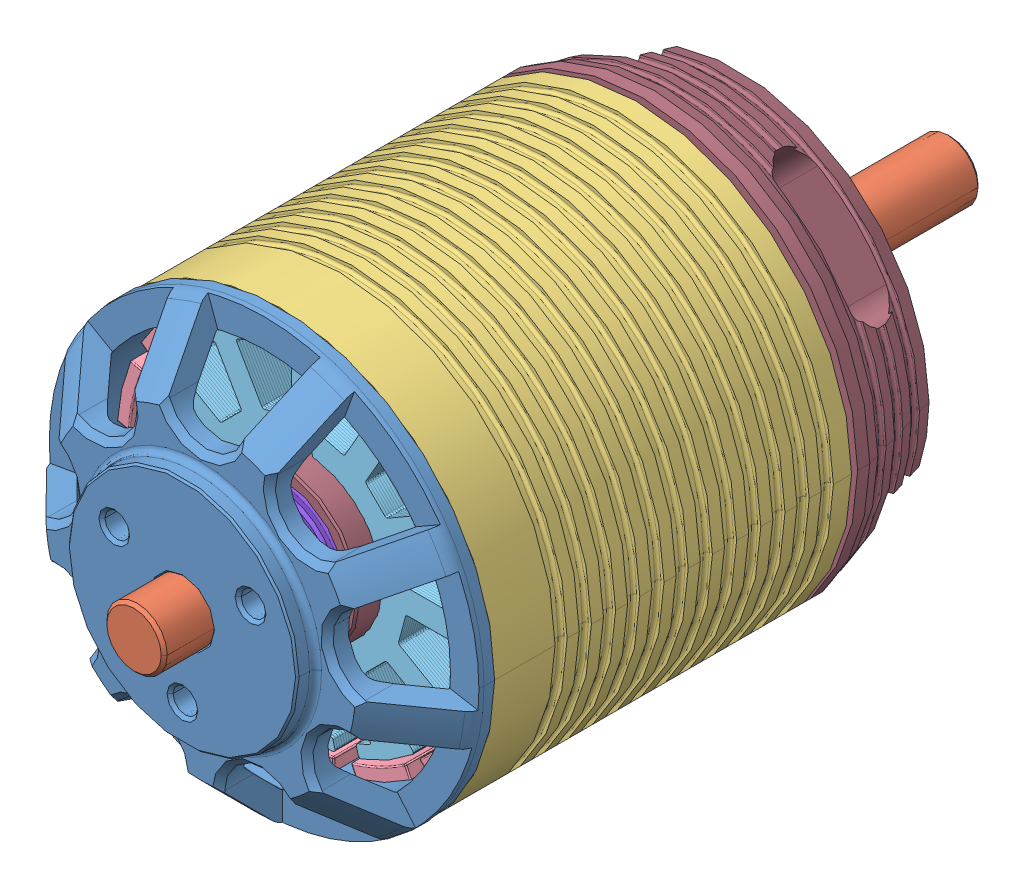
SolidWorks assembly BA-2826-Motor, configuration Default. Lengths in mm.
Overall size (35.6 35.6 67.5).
198 component instances, 15 part files, 0 mates.
Components (placement in the parent):
- BA-2826-Motor(2)^BA-2826-Motor-1: BA-2826-Motor(2)^BA-2826-Motor [Default] at origin size (35.6 35.6 67.5) (virtual)
  - 2826-Rotor-Assem^BA-2826-Motor(2)_BA-2826-Motor-1: 2826-Rotor-Assem^BA-2826-Motor(2)_BA-2826-Motor [Default] at (-10.2441 1.2166 27.3291) size (35.6 35.6 67.5) (virtual)
    - 28mm-Endbell-9^2826-Rotor-Assem_BA-2826-Motor(2)_BA-2826-Motor-1: 28mm-Endbell-9^2826-Rotor-Assem_BA-2826-Motor(2)_BA-2826-Motor [Default] at (-25.4444 8.584 0.3449) size (35.6 35.6 14.5) (virtual)
    - 2826-Shaft^2826-Rotor-Assem_BA-2826-Motor(2)_BA-2826-Motor-1: 2826-Shaft^2826-Rotor-Assem_BA-2826-Motor(2)_BA-2826-Motor [Default] at (-25.4444 8.584 -48.6551) size (5 5 67.5) (virtual)
    - 2826-Fluxring^2826-Rotor-Assem_BA-2826-Motor(2)_BA-2826-Motor-1: 2826-Fluxring^2826-Rotor-Assem_BA-2826-Motor(2)_BA-2826-Motor [Default] at (-25.4444 8.584 -22.6551) size (35.6 35.6 29.5) (virtual)
    - 2826-Magnet^2826-Rotor-Assem_BA-2826-Motor(2)_BA-2826-Motor-1: 2826-Magnet^2826-Rotor-Assem_BA-2826-Motor(2)_BA-2826-Motor [Default] at (-25.4444 8.584 -21.1551) size (5 2.2 26) (virtual)
    - 2826-Magnet^2826-Rotor-Assem_BA-2826-Motor(2)_BA-2826-Motor-2: 2826-Magnet^2826-Rotor-Assem_BA-2826-Motor(2)_BA-2826-Motor [Default] at (-25.4444 8.584 -21.1551) x (0.900969 0.433884 0) z (0 0 1) size (5 2.2 26) (virtual)
    - 2826-Magnet^2826-Rotor-Assem_BA-2826-Motor(2)_BA-2826-Motor-3: 2826-Magnet^2826-Rotor-Assem_BA-2826-Motor(2)_BA-2826-Motor [Default] at (-25.4444 8.584 -21.1551) x (0.62349 0.781831 0) z (0 0 1) size (5 2.2 26) (virtual)
    - 2826-Magnet^2826-Rotor-Assem_BA-2826-Motor(2)_BA-2826-Motor-4: 2826-Magnet^2826-Rotor-Assem_BA-2826-Motor(2)_BA-2826-Motor [Default] at (-25.4444 8.584 -21.1551) x (0.222521 0.974928 0) z (0 0 1) size (5 2.2 26) (virtual)
    - 2826-Magnet^2826-Rotor-Assem_BA-2826-Motor(2)_BA-2826-Motor-5: 2826-Magnet^2826-Rotor-Assem_BA-2826-Motor(2)_BA-2826-Motor [Default] at (-25.4444 8.584 -21.1551) x (-0.222521 0.974928 0) z (0 0 1) size (5 2.2 26) (virtual)
    - 2826-Magnet^2826-Rotor-Assem_BA-2826-Motor(2)_BA-2826-Motor-6: 2826-Magnet^2826-Rotor-Assem_BA-2826-Motor(2)_BA-2826-Motor [Default] at (-25.4444 8.584 -21.1551) x (-0.62349 0.781831 0) z (0 0 1) size (5 2.2 26) (virtual)
    - 2826-Magnet^2826-Rotor-Assem_BA-2826-Motor(2)_BA-2826-Motor-7: 2826-Magnet^2826-Rotor-Assem_BA-2826-Motor(2)_BA-2826-Motor [Default] at (-25.4444 8.584 -21.1551) x (-0.900969 0.433884 0) z (0 0 1) size (5 2.2 26) (virtual)
    - 2826-Magnet^2826-Rotor-Assem_BA-2826-Motor(2)_BA-2826-Motor-8: 2826-Magnet^2826-Rotor-Assem_BA-2826-Motor(2)_BA-2826-Motor [Default] at (-25.4444 8.584 -21.1551) x (-1 0 0) z (0 0 1) size (5 2.2 26) (virtual)
    - 2826-Magnet^2826-Rotor-Assem_BA-2826-Motor(2)_BA-2826-Motor-9: 2826-Magnet^2826-Rotor-Assem_BA-2826-Motor(2)_BA-2826-Motor [Default] at (-25.4444 8.584 -21.1551) x (-0.900969 -0.433884 0) z (0 0 1) size (5 2.2 26) (virtual)
    - 2826-Magnet^2826-Rotor-Assem_BA-2826-Motor(2)_BA-2826-Motor-10: 2826-Magnet^2826-Rotor-Assem_BA-2826-Motor(2)_BA-2826-Motor [Default] at (-25.4444 8.584 -21.1551) x (-0.62349 -0.781831 0) z (0 0 1) size (5 2.2 26) (virtual)
    - 2826-Magnet^2826-Rotor-Assem_BA-2826-Motor(2)_BA-2826-Motor-11: 2826-Magnet^2826-Rotor-Assem_BA-2826-Motor(2)_BA-2826-Motor [Default] at (-25.4444 8.584 -21.1551) x (-0.222521 -0.974928 0) z (0 0 1) size (5 2.2 26) (virtual)
    - 2826-Magnet^2826-Rotor-Assem_BA-2826-Motor(2)_BA-2826-Motor-12: 2826-Magnet^2826-Rotor-Assem_BA-2826-Motor(2)_BA-2826-Motor [Default] at (-25.4444 8.584 -21.1551) x (0.222521 -0.974928 0) z (0 0 1) size (5 2.2 26) (virtual)
    - 2826-Magnet^2826-Rotor-Assem_BA-2826-Motor(2)_BA-2826-Motor-13: 2826-Magnet^2826-Rotor-Assem_BA-2826-Motor(2)_BA-2826-Motor [Default] at (-25.4444 8.584 -21.1551) x (0.62349 -0.781831 0) z (0 0 1) size (5 2.2 26) (virtual)
    - 2826-Magnet^2826-Rotor-Assem_BA-2826-Motor(2)_BA-2826-Motor-14: 2826-Magnet^2826-Rotor-Assem_BA-2826-Motor(2)_BA-2826-Motor [Default] at (-25.4444 8.584 -21.1551) x (0.900969 -0.433884 0) z (0 0 1) size (5 2.2 26) (virtual)
  - 2826-Stator-Mount^BA-2826-Motor(2)_BA-2826-Motor-1: 2826-Stator-Mount^BA-2826-Motor(2)_BA-2826-Motor [Default] at (-12.4646 -13.2477 18.5701) size (35.6 35.6 38.01) (virtual)
    - 28x13x26mm-Stator^2826-Stator-Mount_BA-2826-Motor(2)_BA-2826-Motor-1: 28x13x26mm-Stator^2826-Stator-Mount_BA-2826-Motor(2)_BA-2826-Motor [Default] at (-35.5349 -3.2376 -36.4185) size (28 28 26) (virtual)
      - 28x13x5mm-Stator^28x13x26mm-Stator_2826-Stator-Mount_BA-2826-Motor(2)_BA-2826-Motor-1: 28x13x5mm-Stator^28x13x26mm-Stator_2826-Stator-Mount_BA-2826-Motor(2)_BA-2826-Motor [Default] at (6.5198 12.3714 25.0893) size (28 28 5) (virtual)
        - 28x13x1mm-Stator^28x13x5mm-Stator_28x13x26mm-Stator_2826-Stator-Mount_BA-2826-Motor(2)_BA-2826-Motor-1: 28x13x1mm-Stator^28x13x5mm-Stator_28x13x26mm-Stator_2826-Stator-Mount_BA-2826-Motor(2)_BA-2826-Motor [Default] at (34.0086 1.4103 18.4307) size (28 28 1) (virtual)
          - 28x13-Stator Plate^28x13x1mm-Stator_28x13x5mm-Stator_28x13x26mm-Stator_2826-Stator-Mount_BA-2826-Motor(2)_BA-2826-Motor-1: 28x13-Stator Plate^28x13x1mm-Stator_28x13x5mm-Stator_28x13x26mm-Stator_2826-Stator-Mount_BA-2826-Motor(2)_BA-2826-Motor [Default] at (-28.2175 12.5042 6.2948) size (28 28 0.2) (virtual)
          - 28x13-Stator Plate^28x13x1mm-Stator_28x13x5mm-Stator_28x13x26mm-Stator_2826-Stator-Mount_BA-2826-Motor(2)_BA-2826-Motor-2: 28x13-Stator Plate^28x13x1mm-Stator_28x13x5mm-Stator_28x13x26mm-Stator_2826-Stator-Mount_BA-2826-Motor(2)_BA-2826-Motor [Default] at (-28.2175 12.5042 6.0948) size (28 28 0.2) (virtual)
          - 28x13-Stator Plate^28x13x1mm-Stator_28x13x5mm-Stator_28x13x26mm-Stator_2826-Stator-Mount_BA-2826-Motor(2)_BA-2826-Motor-3: 28x13-Stator Plate^28x13x1mm-Stator_28x13x5mm-Stator_28x13x26mm-Stator_2826-Stator-Mount_BA-2826-Motor(2)_BA-2826-Motor [Default] at (-28.2175 12.5042 5.8948) size (28 28 0.2) (virtual)
          - 28x13-Stator Plate^28x13x1mm-Stator_28x13x5mm-Stator_28x13x26mm-Stator_2826-Stator-Mount_BA-2826-Motor(2)_BA-2826-Motor-4: 28x13-Stator Plate^28x13x1mm-Stator_28x13x5mm-Stator_28x13x26mm-Stator_2826-Stator-Mount_BA-2826-Motor(2)_BA-2826-Motor [Default] at (-28.2175 12.5042 5.6948) size (28 28 0.2) (virtual)
          - 28x13-Stator Plate^28x13x1mm-Stator_28x13x5mm-Stator_28x13x26mm-Stator_2826-Stator-Mount_BA-2826-Motor(2)_BA-2826-Motor-5: 28x13-Stator Plate^28x13x1mm-Stator_28x13x5mm-Stator_28x13x26mm-Stator_2826-Stator-Mount_BA-2826-Motor(2)_BA-2826-Motor [Default] at (-28.2175 12.5042 5.4948) size (28 28 0.2) (virtual)
        - 28x13x1mm-Stator^28x13x5mm-Stator_28x13x26mm-Stator_2826-Stator-Mount_BA-2826-Motor(2)_BA-2826-Motor-2: 28x13x1mm-Stator^28x13x5mm-Stator_28x13x26mm-Stator_2826-Stator-Mount_BA-2826-Motor(2)_BA-2826-Motor [Default] at (34.0086 1.4103 17.4307) size (28 28 1) (virtual)
          - 28x13-Stator Plate^28x13x1mm-Stator_28x13x5mm-Stator_28x13x26mm-Stator_2826-Stator-Mount_BA-2826-Motor(2)_BA-2826-Motor-1: 28x13-Stator Plate^28x13x1mm-Stator_28x13x5mm-Stator_28x13x26mm-Stator_2826-Stator-Mount_BA-2826-Motor(2)_BA-2826-Motor [Default] at (-28.2175 12.5042 6.2948) size (28 28 0.2) (virtual)
          - 28x13-Stator Plate^28x13x1mm-Stator_28x13x5mm-Stator_28x13x26mm-Stator_2826-Stator-Mount_BA-2826-Motor(2)_BA-2826-Motor-2: 28x13-Stator Plate^28x13x1mm-Stator_28x13x5mm-Stator_28x13x26mm-Stator_2826-Stator-Mount_BA-2826-Motor(2)_BA-2826-Motor [Default] at (-28.2175 12.5042 6.0948) size (28 28 0.2) (virtual)
          - 28x13-Stator Plate^28x13x1mm-Stator_28x13x5mm-Stator_28x13x26mm-Stator_2826-Stator-Mount_BA-2826-Motor(2)_BA-2826-Motor-3: 28x13-Stator Plate^28x13x1mm-Stator_28x13x5mm-Stator_28x13x26mm-Stator_2826-Stator-Mount_BA-2826-Motor(2)_BA-2826-Motor [Default] at (-28.2175 12.5042 5.8948) size (28 28 0.2) (virtual)
          - 28x13-Stator Plate^28x13x1mm-Stator_28x13x5mm-Stator_28x13x26mm-Stator_2826-Stator-Mount_BA-2826-Motor(2)_BA-2826-Motor-4: 28x13-Stator Plate^28x13x1mm-Stator_28x13x5mm-Stator_28x13x26mm-Stator_2826-Stator-Mount_BA-2826-Motor(2)_BA-2826-Motor [Default] at (-28.2175 12.5042 5.6948) size (28 28 0.2) (virtual)
          - 28x13-Stator Plate^28x13x1mm-Stator_28x13x5mm-Stator_28x13x26mm-Stator_2826-Stator-Mount_BA-2826-Motor(2)_BA-2826-Motor-5: 28x13-Stator Plate^28x13x1mm-Stator_28x13x5mm-Stator_28x13x26mm-Stator_2826-Stator-Mount_BA-2826-Motor(2)_BA-2826-Motor [Default] at (-28.2175 12.5042 5.4948) size (28 28 0.2) (virtual)
        - 28x13x1mm-Stator^28x13x5mm-Stator_28x13x26mm-Stator_2826-Stator-Mount_BA-2826-Motor(2)_BA-2826-Motor-3: 28x13x1mm-Stator^28x13x5mm-Stator_28x13x26mm-Stator_2826-Stator-Mount_BA-2826-Motor(2)_BA-2826-Motor [Default] at (34.0086 1.4103 16.4307) size (28 28 1) (virtual)
          - 28x13-Stator Plate^28x13x1mm-Stator_28x13x5mm-Stator_28x13x26mm-Stator_2826-Stator-Mount_BA-2826-Motor(2)_BA-2826-Motor-1: 28x13-Stator Plate^28x13x1mm-Stator_28x13x5mm-Stator_28x13x26mm-Stator_2826-Stator-Mount_BA-2826-Motor(2)_BA-2826-Motor [Default] at (-28.2175 12.5042 6.2948) size (28 28 0.2) (virtual)
          - 28x13-Stator Plate^28x13x1mm-Stator_28x13x5mm-Stator_28x13x26mm-Stator_2826-Stator-Mount_BA-2826-Motor(2)_BA-2826-Motor-2: 28x13-Stator Plate^28x13x1mm-Stator_28x13x5mm-Stator_28x13x26mm-Stator_2826-Stator-Mount_BA-2826-Motor(2)_BA-2826-Motor [Default] at (-28.2175 12.5042 6.0948) size (28 28 0.2) (virtual)
          - 28x13-Stator Plate^28x13x1mm-Stator_28x13x5mm-Stator_28x13x26mm-Stator_2826-Stator-Mount_BA-2826-Motor(2)_BA-2826-Motor-3: 28x13-Stator Plate^28x13x1mm-Stator_28x13x5mm-Stator_28x13x26mm-Stator_2826-Stator-Mount_BA-2826-Motor(2)_BA-2826-Motor [Default] at (-28.2175 12.5042 5.8948) size (28 28 0.2) (virtual)
          - 28x13-Stator Plate^28x13x1mm-Stator_28x13x5mm-Stator_28x13x26mm-Stator_2826-Stator-Mount_BA-2826-Motor(2)_BA-2826-Motor-4: 28x13-Stator Plate^28x13x1mm-Stator_28x13x5mm-Stator_28x13x26mm-Stator_2826-Stator-Mount_BA-2826-Motor(2)_BA-2826-Motor [Default] at (-28.2175 12.5042 5.6948) size (28 28 0.2) (virtual)
          - 28x13-Stator Plate^28x13x1mm-Stator_28x13x5mm-Stator_28x13x26mm-Stator_2826-Stator-Mount_BA-2826-Motor(2)_BA-2826-Motor-5: 28x13-Stator Plate^28x13x1mm-Stator_28x13x5mm-Stator_28x13x26mm-Stator_2826-Stator-Mount_BA-2826-Motor(2)_BA-2826-Motor [Default] at (-28.2175 12.5042 5.4948) size (28 28 0.2) (virtual)
        - 28x13x1mm-Stator^28x13x5mm-Stator_28x13x26mm-Stator_2826-Stator-Mount_BA-2826-Motor(2)_BA-2826-Motor-4: 28x13x1mm-Stator^28x13x5mm-Stator_28x13x26mm-Stator_2826-Stator-Mount_BA-2826-Motor(2)_BA-2826-Motor [Default] at (34.0086 1.4103 15.4307) size (28 28 1) (virtual)
          - 28x13-Stator Plate^28x13x1mm-Stator_28x13x5mm-Stator_28x13x26mm-Stator_2826-Stator-Mount_BA-2826-Motor(2)_BA-2826-Motor-1: 28x13-Stator Plate^28x13x1mm-Stator_28x13x5mm-Stator_28x13x26mm-Stator_2826-Stator-Mount_BA-2826-Motor(2)_BA-2826-Motor [Default] at (-28.2175 12.5042 6.2948) size (28 28 0.2) (virtual)
          - 28x13-Stator Plate^28x13x1mm-Stator_28x13x5mm-Stator_28x13x26mm-Stator_2826-Stator-Mount_BA-2826-Motor(2)_BA-2826-Motor-2: 28x13-Stator Plate^28x13x1mm-Stator_28x13x5mm-Stator_28x13x26mm-Stator_2826-Stator-Mount_BA-2826-Motor(2)_BA-2826-Motor [Default] at (-28.2175 12.5042 6.0948) size (28 28 0.2) (virtual)
          - 28x13-Stator Plate^28x13x1mm-Stator_28x13x5mm-Stator_28x13x26mm-Stator_2826-Stator-Mount_BA-2826-Motor(2)_BA-2826-Motor-3: 28x13-Stator Plate^28x13x1mm-Stator_28x13x5mm-Stator_28x13x26mm-Stator_2826-Stator-Mount_BA-2826-Motor(2)_BA-2826-Motor [Default] at (-28.2175 12.5042 5.8948) size (28 28 0.2) (virtual)
          - 28x13-Stator Plate^28x13x1mm-Stator_28x13x5mm-Stator_28x13x26mm-Stator_2826-Stator-Mount_BA-2826-Motor(2)_BA-2826-Motor-4: 28x13-Stator Plate^28x13x1mm-Stator_28x13x5mm-Stator_28x13x26mm-Stator_2826-Stator-Mount_BA-2826-Motor(2)_BA-2826-Motor [Default] at (-28.2175 12.5042 5.6948) size (28 28 0.2) (virtual)
          - 28x13-Stator Plate^28x13x1mm-Stator_28x13x5mm-Stator_28x13x26mm-Stator_2826-Stator-Mount_BA-2826-Motor(2)_BA-2826-Motor-5: 28x13-Stator Plate^28x13x1mm-Stator_28x13x5mm-Stator_28x13x26mm-Stator_2826-Stator-Mount_BA-2826-Motor(2)_BA-2826-Motor [Default] at (-28.2175 12.5042 5.4948) size (28 28 0.2) (virtual)
        - 28x13x1mm-Stator^28x13x5mm-Stator_28x13x26mm-Stator_2826-Stator-Mount_BA-2826-Motor(2)_BA-2826-Motor-5: 28x13x1mm-Stator^28x13x5mm-Stator_28x13x26mm-Stator_2826-Stator-Mount_BA-2826-Motor(2)_BA-2826-Motor [Default] at (34.0086 1.4103 14.4307) size (28 28 1) (virtual)
          - 28x13-Stator Plate^28x13x1mm-Stator_28x13x5mm-Stator_28x13x26mm-Stator_2826-Stator-Mount_BA-2826-Motor(2)_BA-2826-Motor-1: 28x13-Stator Plate^28x13x1mm-Stator_28x13x5mm-Stator_28x13x26mm-Stator_2826-Stator-Mount_BA-2826-Motor(2)_BA-2826-Motor [Default] at (-28.2175 12.5042 6.2948) size (28 28 0.2) (virtual)
          - 28x13-Stator Plate^28x13x1mm-Stator_28x13x5mm-Stator_28x13x26mm-Stator_2826-Stator-Mount_BA-2826-Motor(2)_BA-2826-Motor-2: 28x13-Stator Plate^28x13x1mm-Stator_28x13x5mm-Stator_28x13x26mm-Stator_2826-Stator-Mount_BA-2826-Motor(2)_BA-2826-Motor [Default] at (-28.2175 12.5042 6.0948) size (28 28 0.2) (virtual)
          - 28x13-Stator Plate^28x13x1mm-Stator_28x13x5mm-Stator_28x13x26mm-Stator_2826-Stator-Mount_BA-2826-Motor(2)_BA-2826-Motor-3: 28x13-Stator Plate^28x13x1mm-Stator_28x13x5mm-Stator_28x13x26mm-Stator_2826-Stator-Mount_BA-2826-Motor(2)_BA-2826-Motor [Default] at (-28.2175 12.5042 5.8948) size (28 28 0.2) (virtual)
          - 28x13-Stator Plate^28x13x1mm-Stator_28x13x5mm-Stator_28x13x26mm-Stator_2826-Stator-Mount_BA-2826-Motor(2)_BA-2826-Motor-4: 28x13-Stator Plate^28x13x1mm-Stator_28x13x5mm-Stator_28x13x26mm-Stator_2826-Stator-Mount_BA-2826-Motor(2)_BA-2826-Motor [Default] at (-28.2175 12.5042 5.6948) size (28 28 0.2) (virtual)
          - 28x13-Stator Plate^28x13x1mm-Stator_28x13x5mm-Stator_28x13x26mm-Stator_2826-Stator-Mount_BA-2826-Motor(2)_BA-2826-Motor-5: 28x13-Stator Plate^28x13x1mm-Stator_28x13x5mm-Stator_28x13x26mm-Stator_2826-Stator-Mount_BA-2826-Motor(2)_BA-2826-Motor [Default] at (-28.2175 12.5042 5.4948) size (28 28 0.2) (virtual)
      - 28x13x5mm-Stator^28x13x26mm-Stator_2826-Stator-Mount_BA-2826-Motor(2)_BA-2826-Motor-2: 28x13x5mm-Stator^28x13x26mm-Stator_2826-Stator-Mount_BA-2826-Motor(2)_BA-2826-Motor [Default] at (6.5198 12.3714 20.0893) size (28 28 5) (virtual)
        - 28x13x1mm-Stator^28x13x5mm-Stator_28x13x26mm-Stator_2826-Stator-Mount_BA-2826-Motor(2)_BA-2826-Motor-1: 28x13x1mm-Stator^28x13x5mm-Stator_28x13x26mm-Stator_2826-Stator-Mount_BA-2826-Motor(2)_BA-2826-Motor [Default] at (34.0086 1.4103 18.4307) size (28 28 1) (virtual)
          - 28x13-Stator Plate^28x13x1mm-Stator_28x13x5mm-Stator_28x13x26mm-Stator_2826-Stator-Mount_BA-2826-Motor(2)_BA-2826-Motor-1: 28x13-Stator Plate^28x13x1mm-Stator_28x13x5mm-Stator_28x13x26mm-Stator_2826-Stator-Mount_BA-2826-Motor(2)_BA-2826-Motor [Default] at (-28.2175 12.5042 6.2948) size (28 28 0.2) (virtual)
          - 28x13-Stator Plate^28x13x1mm-Stator_28x13x5mm-Stator_28x13x26mm-Stator_2826-Stator-Mount_BA-2826-Motor(2)_BA-2826-Motor-2: 28x13-Stator Plate^28x13x1mm-Stator_28x13x5mm-Stator_28x13x26mm-Stator_2826-Stator-Mount_BA-2826-Motor(2)_BA-2826-Motor [Default] at (-28.2175 12.5042 6.0948) size (28 28 0.2) (virtual)
          - 28x13-Stator Plate^28x13x1mm-Stator_28x13x5mm-Stator_28x13x26mm-Stator_2826-Stator-Mount_BA-2826-Motor(2)_BA-2826-Motor-3: 28x13-Stator Plate^28x13x1mm-Stator_28x13x5mm-Stator_28x13x26mm-Stator_2826-Stator-Mount_BA-2826-Motor(2)_BA-2826-Motor [Default] at (-28.2175 12.5042 5.8948) size (28 28 0.2) (virtual)
          - 28x13-Stator Plate^28x13x1mm-Stator_28x13x5mm-Stator_28x13x26mm-Stator_2826-Stator-Mount_BA-2826-Motor(2)_BA-2826-Motor-4: 28x13-Stator Plate^28x13x1mm-Stator_28x13x5mm-Stator_28x13x26mm-Stator_2826-Stator-Mount_BA-2826-Motor(2)_BA-2826-Motor [Default] at (-28.2175 12.5042 5.6948) size (28 28 0.2) (virtual)
          - 28x13-Stator Plate^28x13x1mm-Stator_28x13x5mm-Stator_28x13x26mm-Stator_2826-Stator-Mount_BA-2826-Motor(2)_BA-2826-Motor-5: 28x13-Stator Plate^28x13x1mm-Stator_28x13x5mm-Stator_28x13x26mm-Stator_2826-Stator-Mount_BA-2826-Motor(2)_BA-2826-Motor [Default] at (-28.2175 12.5042 5.4948) size (28 28 0.2) (virtual)
        - 28x13x1mm-Stator^28x13x5mm-Stator_28x13x26mm-Stator_2826-Stator-Mount_BA-2826-Motor(2)_BA-2826-Motor-2: 28x13x1mm-Stator^28x13x5mm-Stator_28x13x26mm-Stator_2826-Stator-Mount_BA-2826-Motor(2)_BA-2826-Motor [Default] at (34.0086 1.4103 17.4307) size (28 28 1) (virtual)
          - 28x13-Stator Plate^28x13x1mm-Stator_28x13x5mm-Stator_28x13x26mm-Stator_2826-Stator-Mount_BA-2826-Motor(2)_BA-2826-Motor-1: 28x13-Stator Plate^28x13x1mm-Stator_28x13x5mm-Stator_28x13x26mm-Stator_2826-Stator-Mount_BA-2826-Motor(2)_BA-2826-Motor [Default] at (-28.2175 12.5042 6.2948) size (28 28 0.2) (virtual)
          - 28x13-Stator Plate^28x13x1mm-Stator_28x13x5mm-Stator_28x13x26mm-Stator_2826-Stator-Mount_BA-2826-Motor(2)_BA-2826-Motor-2: 28x13-Stator Plate^28x13x1mm-Stator_28x13x5mm-Stator_28x13x26mm-Stator_2826-Stator-Mount_BA-2826-Motor(2)_BA-2826-Motor [Default] at (-28.2175 12.5042 6.0948) size (28 28 0.2) (virtual)
          - 28x13-Stator Plate^28x13x1mm-Stator_28x13x5mm-Stator_28x13x26mm-Stator_2826-Stator-Mount_BA-2826-Motor(2)_BA-2826-Motor-3: 28x13-Stator Plate^28x13x1mm-Stator_28x13x5mm-Stator_28x13x26mm-Stator_2826-Stator-Mount_BA-2826-Motor(2)_BA-2826-Motor [Default] at (-28.2175 12.5042 5.8948) size (28 28 0.2) (virtual)
          - 28x13-Stator Plate^28x13x1mm-Stator_28x13x5mm-Stator_28x13x26mm-Stator_2826-Stator-Mount_BA-2826-Motor(2)_BA-2826-Motor-4: 28x13-Stator Plate^28x13x1mm-Stator_28x13x5mm-Stator_28x13x26mm-Stator_2826-Stator-Mount_BA-2826-Motor(2)_BA-2826-Motor [Default] at (-28.2175 12.5042 5.6948) size (28 28 0.2) (virtual)
          - 28x13-Stator Plate^28x13x1mm-Stator_28x13x5mm-Stator_28x13x26mm-Stator_2826-Stator-Mount_BA-2826-Motor(2)_BA-2826-Motor-5: 28x13-Stator Plate^28x13x1mm-Stator_28x13x5mm-Stator_28x13x26mm-Stator_2826-Stator-Mount_BA-2826-Motor(2)_BA-2826-Motor [Default] at (-28.2175 12.5042 5.4948) size (28 28 0.2) (virtual)
        - 28x13x1mm-Stator^28x13x5mm-Stator_28x13x26mm-Stator_2826-Stator-Mount_BA-2826-Motor(2)_BA-2826-Motor-3: 28x13x1mm-Stator^28x13x5mm-Stator_28x13x26mm-Stator_2826-Stator-Mount_BA-2826-Motor(2)_BA-2826-Motor [Default] at (34.0086 1.4103 16.4307) size (28 28 1) (virtual)
          - 28x13-Stator Plate^28x13x1mm-Stator_28x13x5mm-Stator_28x13x26mm-Stator_2826-Stator-Mount_BA-2826-Motor(2)_BA-2826-Motor-1: 28x13-Stator Plate^28x13x1mm-Stator_28x13x5mm-Stator_28x13x26mm-Stator_2826-Stator-Mount_BA-2826-Motor(2)_BA-2826-Motor [Default] at (-28.2175 12.5042 6.2948) size (28 28 0.2) (virtual)
          - 28x13-Stator Plate^28x13x1mm-Stator_28x13x5mm-Stator_28x13x26mm-Stator_2826-Stator-Mount_BA-2826-Motor(2)_BA-2826-Motor-2: 28x13-Stator Plate^28x13x1mm-Stator_28x13x5mm-Stator_28x13x26mm-Stator_2826-Stator-Mount_BA-2826-Motor(2)_BA-2826-Motor [Default] at (-28.2175 12.5042 6.0948) size (28 28 0.2) (virtual)
          - 28x13-Stator Plate^28x13x1mm-Stator_28x13x5mm-Stator_28x13x26mm-Stator_2826-Stator-Mount_BA-2826-Motor(2)_BA-2826-Motor-3: 28x13-Stator Plate^28x13x1mm-Stator_28x13x5mm-Stator_28x13x26mm-Stator_2826-Stator-Mount_BA-2826-Motor(2)_BA-2826-Motor [Default] at (-28.2175 12.5042 5.8948) size (28 28 0.2) (virtual)
          - 28x13-Stator Plate^28x13x1mm-Stator_28x13x5mm-Stator_28x13x26mm-Stator_2826-Stator-Mount_BA-2826-Motor(2)_BA-2826-Motor-4: 28x13-Stator Plate^28x13x1mm-Stator_28x13x5mm-Stator_28x13x26mm-Stator_2826-Stator-Mount_BA-2826-Motor(2)_BA-2826-Motor [Default] at (-28.2175 12.5042 5.6948) size (28 28 0.2) (virtual)
          - 28x13-Stator Plate^28x13x1mm-Stator_28x13x5mm-Stator_28x13x26mm-Stator_2826-Stator-Mount_BA-2826-Motor(2)_BA-2826-Motor-5: 28x13-Stator Plate^28x13x1mm-Stator_28x13x5mm-Stator_28x13x26mm-Stator_2826-Stator-Mount_BA-2826-Motor(2)_BA-2826-Motor [Default] at (-28.2175 12.5042 5.4948) size (28 28 0.2) (virtual)
        - 28x13x1mm-Stator^28x13x5mm-Stator_28x13x26mm-Stator_2826-Stator-Mount_BA-2826-Motor(2)_BA-2826-Motor-4: 28x13x1mm-Stator^28x13x5mm-Stator_28x13x26mm-Stator_2826-Stator-Mount_BA-2826-Motor(2)_BA-2826-Motor [Default] at (34.0086 1.4103 15.4307) size (28 28 1) (virtual)
          - 28x13-Stator Plate^28x13x1mm-Stator_28x13x5mm-Stator_28x13x26mm-Stator_2826-Stator-Mount_BA-2826-Motor(2)_BA-2826-Motor-1: 28x13-Stator Plate^28x13x1mm-Stator_28x13x5mm-Stator_28x13x26mm-Stator_2826-Stator-Mount_BA-2826-Motor(2)_BA-2826-Motor [Default] at (-28.2175 12.5042 6.2948) size (28 28 0.2) (virtual)
          - 28x13-Stator Plate^28x13x1mm-Stator_28x13x5mm-Stator_28x13x26mm-Stator_2826-Stator-Mount_BA-2826-Motor(2)_BA-2826-Motor-2: 28x13-Stator Plate^28x13x1mm-Stator_28x13x5mm-Stator_28x13x26mm-Stator_2826-Stator-Mount_BA-2826-Motor(2)_BA-2826-Motor [Default] at (-28.2175 12.5042 6.0948) size (28 28 0.2) (virtual)
          - 28x13-Stator Plate^28x13x1mm-Stator_28x13x5mm-Stator_28x13x26mm-Stator_2826-Stator-Mount_BA-2826-Motor(2)_BA-2826-Motor-3: 28x13-Stator Plate^28x13x1mm-Stator_28x13x5mm-Stator_28x13x26mm-Stator_2826-Stator-Mount_BA-2826-Motor(2)_BA-2826-Motor [Default] at (-28.2175 12.5042 5.8948) size (28 28 0.2) (virtual)
          - 28x13-Stator Plate^28x13x1mm-Stator_28x13x5mm-Stator_28x13x26mm-Stator_2826-Stator-Mount_BA-2826-Motor(2)_BA-2826-Motor-4: 28x13-Stator Plate^28x13x1mm-Stator_28x13x5mm-Stator_28x13x26mm-Stator_2826-Stator-Mount_BA-2826-Motor(2)_BA-2826-Motor [Default] at (-28.2175 12.5042 5.6948) size (28 28 0.2) (virtual)
          - 28x13-Stator Plate^28x13x1mm-Stator_28x13x5mm-Stator_28x13x26mm-Stator_2826-Stator-Mount_BA-2826-Motor(2)_BA-2826-Motor-5: 28x13-Stator Plate^28x13x1mm-Stator_28x13x5mm-Stator_28x13x26mm-Stator_2826-Stator-Mount_BA-2826-Motor(2)_BA-2826-Motor [Default] at (-28.2175 12.5042 5.4948) size (28 28 0.2) (virtual)
        - 28x13x1mm-Stator^28x13x5mm-Stator_28x13x26mm-Stator_2826-Stator-Mount_BA-2826-Motor(2)_BA-2826-Motor-5: 28x13x1mm-Stator^28x13x5mm-Stator_28x13x26mm-Stator_2826-Stator-Mount_BA-2826-Motor(2)_BA-2826-Motor [Default] at (34.0086 1.4103 14.4307) size (28 28 1) (virtual)
          - 28x13-Stator Plate^28x13x1mm-Stator_28x13x5mm-Stator_28x13x26mm-Stator_2826-Stator-Mount_BA-2826-Motor(2)_BA-2826-Motor-1: 28x13-Stator Plate^28x13x1mm-Stator_28x13x5mm-Stator_28x13x26mm-Stator_2826-Stator-Mount_BA-2826-Motor(2)_BA-2826-Motor [Default] at (-28.2175 12.5042 6.2948) size (28 28 0.2) (virtual)
          - 28x13-Stator Plate^28x13x1mm-Stator_28x13x5mm-Stator_28x13x26mm-Stator_2826-Stator-Mount_BA-2826-Motor(2)_BA-2826-Motor-2: 28x13-Stator Plate^28x13x1mm-Stator_28x13x5mm-Stator_28x13x26mm-Stator_2826-Stator-Mount_BA-2826-Motor(2)_BA-2826-Motor [Default] at (-28.2175 12.5042 6.0948) size (28 28 0.2) (virtual)
          - 28x13-Stator Plate^28x13x1mm-Stator_28x13x5mm-Stator_28x13x26mm-Stator_2826-Stator-Mount_BA-2826-Motor(2)_BA-2826-Motor-3: 28x13-Stator Plate^28x13x1mm-Stator_28x13x5mm-Stator_28x13x26mm-Stator_2826-Stator-Mount_BA-2826-Motor(2)_BA-2826-Motor [Default] at (-28.2175 12.5042 5.8948) size (28 28 0.2) (virtual)
          - 28x13-Stator Plate^28x13x1mm-Stator_28x13x5mm-Stator_28x13x26mm-Stator_2826-Stator-Mount_BA-2826-Motor(2)_BA-2826-Motor-4: 28x13-Stator Plate^28x13x1mm-Stator_28x13x5mm-Stator_28x13x26mm-Stator_2826-Stator-Mount_BA-2826-Motor(2)_BA-2826-Motor [Default] at (-28.2175 12.5042 5.6948) size (28 28 0.2) (virtual)
          - 28x13-Stator Plate^28x13x1mm-Stator_28x13x5mm-Stator_28x13x26mm-Stator_2826-Stator-Mount_BA-2826-Motor(2)_BA-2826-Motor-5: 28x13-Stator Plate^28x13x1mm-Stator_28x13x5mm-Stator_28x13x26mm-Stator_2826-Stator-Mount_BA-2826-Motor(2)_BA-2826-Motor [Default] at (-28.2175 12.5042 5.4948) size (28 28 0.2) (virtual)
      - 28x13x5mm-Stator^28x13x26mm-Stator_2826-Stator-Mount_BA-2826-Motor(2)_BA-2826-Motor-3: 28x13x5mm-Stator^28x13x26mm-Stator_2826-Stator-Mount_BA-2826-Motor(2)_BA-2826-Motor [Default] at (6.5198 12.3714 15.0893) size (28 28 5) (virtual)
        - 28x13x1mm-Stator^28x13x5mm-Stator_28x13x26mm-Stator_2826-Stator-Mount_BA-2826-Motor(2)_BA-2826-Motor-1: 28x13x1mm-Stator^28x13x5mm-Stator_28x13x26mm-Stator_2826-Stator-Mount_BA-2826-Motor(2)_BA-2826-Motor [Default] at (34.0086 1.4103 18.4307) size (28 28 1) (virtual)
          - 28x13-Stator Plate^28x13x1mm-Stator_28x13x5mm-Stator_28x13x26mm-Stator_2826-Stator-Mount_BA-2826-Motor(2)_BA-2826-Motor-1: 28x13-Stator Plate^28x13x1mm-Stator_28x13x5mm-Stator_28x13x26mm-Stator_2826-Stator-Mount_BA-2826-Motor(2)_BA-2826-Motor [Default] at (-28.2175 12.5042 6.2948) size (28 28 0.2) (virtual)
          - 28x13-Stator Plate^28x13x1mm-Stator_28x13x5mm-Stator_28x13x26mm-Stator_2826-Stator-Mount_BA-2826-Motor(2)_BA-2826-Motor-2: 28x13-Stator Plate^28x13x1mm-Stator_28x13x5mm-Stator_28x13x26mm-Stator_2826-Stator-Mount_BA-2826-Motor(2)_BA-2826-Motor [Default] at (-28.2175 12.5042 6.0948) size (28 28 0.2) (virtual)
          - 28x13-Stator Plate^28x13x1mm-Stator_28x13x5mm-Stator_28x13x26mm-Stator_2826-Stator-Mount_BA-2826-Motor(2)_BA-2826-Motor-3: 28x13-Stator Plate^28x13x1mm-Stator_28x13x5mm-Stator_28x13x26mm-Stator_2826-Stator-Mount_BA-2826-Motor(2)_BA-2826-Motor [Default] at (-28.2175 12.5042 5.8948) size (28 28 0.2) (virtual)
          - 28x13-Stator Plate^28x13x1mm-Stator_28x13x5mm-Stator_28x13x26mm-Stator_2826-Stator-Mount_BA-2826-Motor(2)_BA-2826-Motor-4: 28x13-Stator Plate^28x13x1mm-Stator_28x13x5mm-Stator_28x13x26mm-Stator_2826-Stator-Mount_BA-2826-Motor(2)_BA-2826-Motor [Default] at (-28.2175 12.5042 5.6948) size (28 28 0.2) (virtual)
          - 28x13-Stator Plate^28x13x1mm-Stator_28x13x5mm-Stator_28x13x26mm-Stator_2826-Stator-Mount_BA-2826-Motor(2)_BA-2826-Motor-5: 28x13-Stator Plate^28x13x1mm-Stator_28x13x5mm-Stator_28x13x26mm-Stator_2826-Stator-Mount_BA-2826-Motor(2)_BA-2826-Motor [Default] at (-28.2175 12.5042 5.4948) size (28 28 0.2) (virtual)
        - 28x13x1mm-Stator^28x13x5mm-Stator_28x13x26mm-Stator_2826-Stator-Mount_BA-2826-Motor(2)_BA-2826-Motor-2: 28x13x1mm-Stator^28x13x5mm-Stator_28x13x26mm-Stator_2826-Stator-Mount_BA-2826-Motor(2)_BA-2826-Motor [Default] at (34.0086 1.4103 17.4307) size (28 28 1) (virtual)
          - 28x13-Stator Plate^28x13x1mm-Stator_28x13x5mm-Stator_28x13x26mm-Stator_2826-Stator-Mount_BA-2826-Motor(2)_BA-2826-Motor-1: 28x13-Stator Plate^28x13x1mm-Stator_28x13x5mm-Stator_28x13x26mm-Stator_2826-Stator-Mount_BA-2826-Motor(2)_BA-2826-Motor [Default] at (-28.2175 12.5042 6.2948) size (28 28 0.2) (virtual)
          - 28x13-Stator Plate^28x13x1mm-Stator_28x13x5mm-Stator_28x13x26mm-Stator_2826-Stator-Mount_BA-2826-Motor(2)_BA-2826-Motor-2: 28x13-Stator Plate^28x13x1mm-Stator_28x13x5mm-Stator_28x13x26mm-Stator_2826-Stator-Mount_BA-2826-Motor(2)_BA-2826-Motor [Default] at (-28.2175 12.5042 6.0948) size (28 28 0.2) (virtual)
          - 28x13-Stator Plate^28x13x1mm-Stator_28x13x5mm-Stator_28x13x26mm-Stator_2826-Stator-Mount_BA-2826-Motor(2)_BA-2826-Motor-3: 28x13-Stator Plate^28x13x1mm-Stator_28x13x5mm-Stator_28x13x26mm-Stator_2826-Stator-Mount_BA-2826-Motor(2)_BA-2826-Motor [Default] at (-28.2175 12.5042 5.8948) size (28 28 0.2) (virtual)
          - 28x13-Stator Plate^28x13x1mm-Stator_28x13x5mm-Stator_28x13x26mm-Stator_2826-Stator-Mount_BA-2826-Motor(2)_BA-2826-Motor-4: 28x13-Stator Plate^28x13x1mm-Stator_28x13x5mm-Stator_28x13x26mm-Stator_2826-Stator-Mount_BA-2826-Motor(2)_BA-2826-Motor [Default] at (-28.2175 12.5042 5.6948) size (28 28 0.2) (virtual)
          - 28x13-Stator Plate^28x13x1mm-Stator_28x13x5mm-Stator_28x13x26mm-Stator_2826-Stator-Mount_BA-2826-Motor(2)_BA-2826-Motor-5: 28x13-Stator Plate^28x13x1mm-Stator_28x13x5mm-Stator_28x13x26mm-Stator_2826-Stator-Mount_BA-2826-Motor(2)_BA-2826-Motor [Default] at (-28.2175 12.5042 5.4948) size (28 28 0.2) (virtual)
        - 28x13x1mm-Stator^28x13x5mm-Stator_28x13x26mm-Stator_2826-Stator-Mount_BA-2826-Motor(2)_BA-2826-Motor-3: 28x13x1mm-Stator^28x13x5mm-Stator_28x13x26mm-Stator_2826-Stator-Mount_BA-2826-Motor(2)_BA-2826-Motor [Default] at (34.0086 1.4103 16.4307) size (28 28 1) (virtual)
          - 28x13-Stator Plate^28x13x1mm-Stator_28x13x5mm-Stator_28x13x26mm-Stator_2826-Stator-Mount_BA-2826-Motor(2)_BA-2826-Motor-1: 28x13-Stator Plate^28x13x1mm-Stator_28x13x5mm-Stator_28x13x26mm-Stator_2826-Stator-Mount_BA-2826-Motor(2)_BA-2826-Motor [Default] at (-28.2175 12.5042 6.2948) size (28 28 0.2) (virtual)
          - 28x13-Stator Plate^28x13x1mm-Stator_28x13x5mm-Stator_28x13x26mm-Stator_2826-Stator-Mount_BA-2826-Motor(2)_BA-2826-Motor-2: 28x13-Stator Plate^28x13x1mm-Stator_28x13x5mm-Stator_28x13x26mm-Stator_2826-Stator-Mount_BA-2826-Motor(2)_BA-2826-Motor [Default] at (-28.2175 12.5042 6.0948) size (28 28 0.2) (virtual)
          - 28x13-Stator Plate^28x13x1mm-Stator_28x13x5mm-Stator_28x13x26mm-Stator_2826-Stator-Mount_BA-2826-Motor(2)_BA-2826-Motor-3: 28x13-Stator Plate^28x13x1mm-Stator_28x13x5mm-Stator_28x13x26mm-Stator_2826-Stator-Mount_BA-2826-Motor(2)_BA-2826-Motor [Default] at (-28.2175 12.5042 5.8948) size (28 28 0.2) (virtual)
          - 28x13-Stator Plate^28x13x1mm-Stator_28x13x5mm-Stator_28x13x26mm-Stator_2826-Stator-Mount_BA-2826-Motor(2)_BA-2826-Motor-4: 28x13-Stator Plate^28x13x1mm-Stator_28x13x5mm-Stator_28x13x26mm-Stator_2826-Stator-Mount_BA-2826-Motor(2)_BA-2826-Motor [Default] at (-28.2175 12.5042 5.6948) size (28 28 0.2) (virtual)
          - 28x13-Stator Plate^28x13x1mm-Stator_28x13x5mm-Stator_28x13x26mm-Stator_2826-Stator-Mount_BA-2826-Motor(2)_BA-2826-Motor-5: 28x13-Stator Plate^28x13x1mm-Stator_28x13x5mm-Stator_28x13x26mm-Stator_2826-Stator-Mount_BA-2826-Motor(2)_BA-2826-Motor [Default] at (-28.2175 12.5042 5.4948) size (28 28 0.2) (virtual)
        - 28x13x1mm-Stator^28x13x5mm-Stator_28x13x26mm-Stator_2826-Stator-Mount_BA-2826-Motor(2)_BA-2826-Motor-4: 28x13x1mm-Stator^28x13x5mm-Stator_28x13x26mm-Stator_2826-Stator-Mount_BA-2826-Motor(2)_BA-2826-Motor [Default] at (34.0086 1.4103 15.4307) size (28 28 1) (virtual)
          - 28x13-Stator Plate^28x13x1mm-Stator_28x13x5mm-Stator_28x13x26mm-Stator_2826-Stator-Mount_BA-2826-Motor(2)_BA-2826-Motor-1: 28x13-Stator Plate^28x13x1mm-Stator_28x13x5mm-Stator_28x13x26mm-Stator_2826-Stator-Mount_BA-2826-Motor(2)_BA-2826-Motor [Default] at (-28.2175 12.5042 6.2948) size (28 28 0.2) (virtual)
          - 28x13-Stator Plate^28x13x1mm-Stator_28x13x5mm-Stator_28x13x26mm-Stator_2826-Stator-Mount_BA-2826-Motor(2)_BA-2826-Motor-2: 28x13-Stator Plate^28x13x1mm-Stator_28x13x5mm-Stator_28x13x26mm-Stator_2826-Stator-Mount_BA-2826-Motor(2)_BA-2826-Motor [Default] at (-28.2175 12.5042 6.0948) size (28 28 0.2) (virtual)
          - 28x13-Stator Plate^28x13x1mm-Stator_28x13x5mm-Stator_28x13x26mm-Stator_2826-Stator-Mount_BA-2826-Motor(2)_BA-2826-Motor-3: 28x13-Stator Plate^28x13x1mm-Stator_28x13x5mm-Stator_28x13x26mm-Stator_2826-Stator-Mount_BA-2826-Motor(2)_BA-2826-Motor [Default] at (-28.2175 12.5042 5.8948) size (28 28 0.2) (virtual)
          - 28x13-Stator Plate^28x13x1mm-Stator_28x13x5mm-Stator_28x13x26mm-Stator_2826-Stator-Mount_BA-2826-Motor(2)_BA-2826-Motor-4: 28x13-Stator Plate^28x13x1mm-Stator_28x13x5mm-Stator_28x13x26mm-Stator_2826-Stator-Mount_BA-2826-Motor(2)_BA-2826-Motor [Default] at (-28.2175 12.5042 5.6948) size (28 28 0.2) (virtual)
          - 28x13-Stator Plate^28x13x1mm-Stator_28x13x5mm-Stator_28x13x26mm-Stator_2826-Stator-Mount_BA-2826-Motor(2)_BA-2826-Motor-5: 28x13-Stator Plate^28x13x1mm-Stator_28x13x5mm-Stator_28x13x26mm-Stator_2826-Stator-Mount_BA-2826-Motor(2)_BA-2826-Motor [Default] at (-28.2175 12.5042 5.4948) size (28 28 0.2) (virtual)
        - 28x13x1mm-Stator^28x13x5mm-Stator_28x13x26mm-Stator_2826-Stator-Mount_BA-2826-Motor(2)_BA-2826-Motor-5: 28x13x1mm-Stator^28x13x5mm-Stator_28x13x26mm-Stator_2826-Stator-Mount_BA-2826-Motor(2)_BA-2826-Motor [Default] at (34.0086 1.4103 14.4307) size (28 28 1) (virtual)
          - 28x13-Stator Plate^28x13x1mm-Stator_28x13x5mm-Stator_28x13x26mm-Stator_2826-Stator-Mount_BA-2826-Motor(2)_BA-2826-Motor-1: 28x13-Stator Plate^28x13x1mm-Stator_28x13x5mm-Stator_28x13x26mm-Stator_2826-Stator-Mount_BA-2826-Motor(2)_BA-2826-Motor [Default] at (-28.2175 12.5042 6.2948) size (28 28 0.2) (virtual)
          - 28x13-Stator Plate^28x13x1mm-Stator_28x13x5mm-Stator_28x13x26mm-Stator_2826-Stator-Mount_BA-2826-Motor(2)_BA-2826-Motor-2: 28x13-Stator Plate^28x13x1mm-Stator_28x13x5mm-Stator_28x13x26mm-Stator_2826-Stator-Mount_BA-2826-Motor(2)_BA-2826-Motor [Default] at (-28.2175 12.5042 6.0948) size (28 28 0.2) (virtual)
          - 28x13-Stator Plate^28x13x1mm-Stator_28x13x5mm-Stator_28x13x26mm-Stator_2826-Stator-Mount_BA-2826-Motor(2)_BA-2826-Motor-3: 28x13-Stator Plate^28x13x1mm-Stator_28x13x5mm-Stator_28x13x26mm-Stator_2826-Stator-Mount_BA-2826-Motor(2)_BA-2826-Motor [Default] at (-28.2175 12.5042 5.8948) size (28 28 0.2) (virtual)
          - 28x13-Stator Plate^28x13x1mm-Stator_28x13x5mm-Stator_28x13x26mm-Stator_2826-Stator-Mount_BA-2826-Motor(2)_BA-2826-Motor-4: 28x13-Stator Plate^28x13x1mm-Stator_28x13x5mm-Stator_28x13x26mm-Stator_2826-Stator-Mount_BA-2826-Motor(2)_BA-2826-Motor [Default] at (-28.2175 12.5042 5.6948) size (28 28 0.2) (virtual)
          - 28x13-Stator Plate^28x13x1mm-Stator_28x13x5mm-Stator_28x13x26mm-Stator_2826-Stator-Mount_BA-2826-Motor(2)_BA-2826-Motor-5: 28x13-Stator Plate^28x13x1mm-Stator_28x13x5mm-Stator_28x13x26mm-Stator_2826-Stator-Mount_BA-2826-Motor(2)_BA-2826-Motor [Default] at (-28.2175 12.5042 5.4948) size (28 28 0.2) (virtual)
